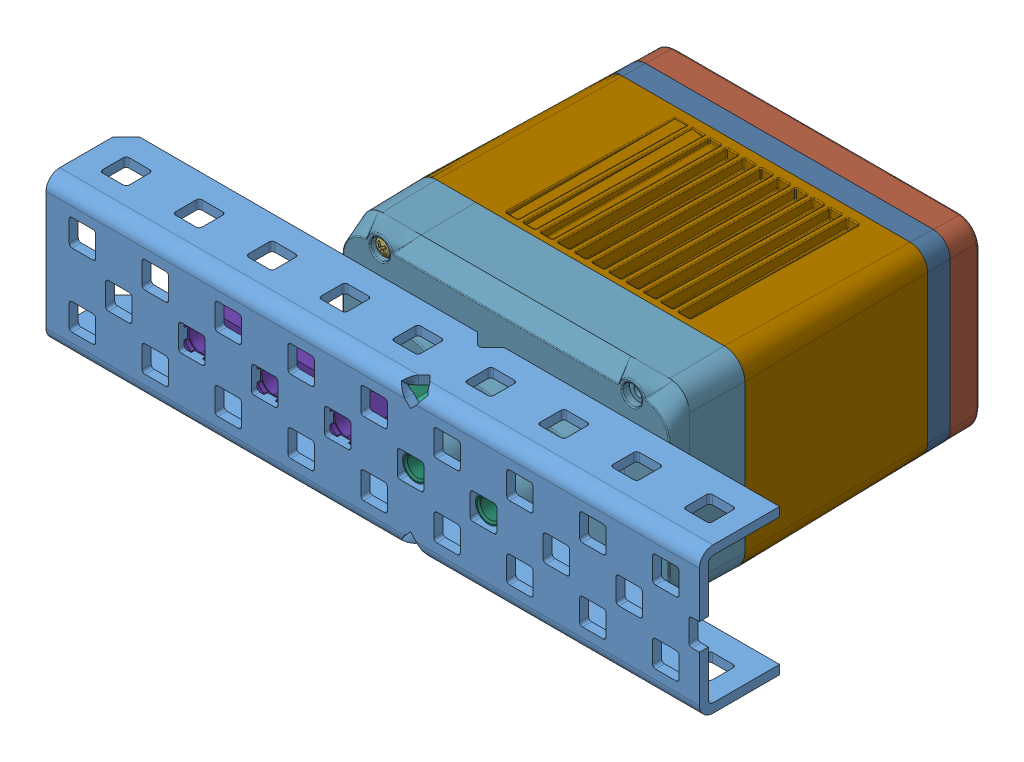
SolidWorks assembly MotorMount1, configuration Default. Lengths in mm.
Overall size (113.79 35.33 73.19).
29 component instances, 17 part files, 6 mates.
Components (placement in the parent):
- 1x2x1x9 Aluminum C-Channel-1: 1x2x1x9 Aluminum C-Channel [Default] at (207.6372 62.1851 92.5266) size (113.79 25.41 13.97)
- V5 Smart Motor (276-4840) 2-1: V5 Smart Motor (276-4840) 2 [Default] at (48.8872 62.1851 46.7518) x (-1 0 0) z (0 0 1) size (59.01 35.33 72.31)
  - V5 Smart Motor (276-4840) 2.step-1: V5 Smart Motor (276-4840) 2.step [Default] at origin size (59.01 35.33 72.31)
    - 276-4840-900 Rev6_Instruction.step-1: 276-4840-900 Rev6_Instruction.step [Default] at (-14.3 0 -17.2) size (52.79 15.94 38.15)
      - 276-4840-901 Rev6.step-1: 276-4840-901 Rev6.step [Default] at (10.75 -10.05 17.8) x (-1 0 0) z (0 0 1) size (49.9 1.6 38.15)
      - 276-4840-902 Rev2.step-1: 276-4840-902 Rev2.step [Default] at (31.25 -9.25 6.2) x (0 0 -1) z (0 -1 0) size (10.35 11.39 15.94)
      - 276-4840-022 Rev4.step-1: 276-4840-022 Rev4.step [Default] at (31.25 -9.25 6.2) x (0 0 -1) z (1 0 0) size (10.26 9.1 5.51)
    - 276-4840-110 Rev10_Instruction.step-1: 276-4840-110 Rev10_Instruction.step [Default] at (12.7 0 14.7) size (35.33 35.33 31.1)
      - 276-4840-061 Rev7_Ring_Gear_Fixed01 .6 Rev3.step-1: 276-4840-061 Rev7_Ring_Gear_Fixed01 .6 Rev3.step [Default] at origin size (28.79 28.39 24.6)
      - 276-4840-018 Rev6.step-1: 276-4840-018 Rev6.step [Default] at (0 0 6.7) x (-0.483174 0.875524 0) z (0 0 1) size (26 26 12.3)
      - 276-4840-059 Rev2.step-1: 276-4840-059 Rev2.step [Default] at (0 0 10.3) size (28.4 28.4 8.5)
      - 276-4840-062 Rev1.step-1: 276-4840-062 Rev1.step [Default] at (-12.1353 8.8168 12.3) x (0.956835 -0.290632 0) z (-0.290632 -0.956835 0) size (3.2 6.56 3.2)
      - 276-4840-062 Rev1.step-2: 276-4840-062 Rev1.step [Default] at (12.1353 8.8168 12.3) x (0.978427 0.206591 0) z (0.206591 -0.978427 0) size (3.2 6.56 3.2)
      - 276-4840-062 Rev1.step-3: 276-4840-062 Rev1.step [Default] at (-12.1353 -8.8168 12.3) x (0.72563 0.688086 0) z (0.688086 -0.72563 0) size (3.2 6.56 3.2)
    - 276-4840-001 Rev38.step-1: 276-4840-001 Rev38.step [Default] at origin size (57.3 33 46.9)
    - 276-4840-005 Rev27.step-1: 276-4840-005 Rev27.step [Default] at (0 0 -17.95) size (56.17 31.87 12.9)
    - 276-4840-004 Rev16.step-1: 276-4840-004 Rev16.step [Default] at (0 0 -19.2) size (56.01 31.71 9.21)
    - 276-4840-015 Rev7.step-1: 276-4840-015 Rev7.step [Default] at (-21.95 14 27.9) x (-0.85131 -0.524663 0) z (-0.524663 0.85131 0) size (3.2 17.55 3.2)
    - 276-4840-015 Rev7.step-2: 276-4840-015 Rev7.step [Default] at (21.95 -14 27.9) x (-0.777574 -0.628792 0) z (-0.628792 0.777574 0) size (3.2 17.55 3.2)
    - 276-4840-015 Rev7.step-3: 276-4840-015 Rev7.step [Default] at (21.95 14 27.9) x (0.476859 0.87898 0) z (0.87898 -0.476859 0) size (3.2 17.55 3.2)
    - 276-4840-009 Rev3.step-1: 276-4840-009 Rev3.step [Default] at (25.45 13.5 15.7) x (0.19987 -0.979823 0) z (-0.979823 -0.19987 0) size (3.4 41.31 4.34)
    - 276-4840-009 Rev3.step-2: 276-4840-009 Rev3.step [Default] at (-25.45 -13.5 15.7) x (-0.998855 0.047836 0) z (0.047836 0.998855 0) size (3.4 41.31 4.34)
    - 276-4840-009 Rev3.step-3: 276-4840-009 Rev3.step [Default] at (25.45 -13.5 15.7) x (-0.975374 0.220559 0) z (0.220559 0.975374 0) size (3.4 41.31 4.34)
    - 276-4840-009 Rev3.step-4: 276-4840-009 Rev3.step [Default] at (-25.45 13.5 15.7) x (-0.922256 0.38658 0) z (0.38658 0.922256 0) size (3.4 41.31 4.34)
    - 276-4840-003 Rev27.step-1: 276-4840-003 Rev27.step [Default] at (0 0 16.2) size (57.3 33 28.01)
    - 276-4840-043 Rev8.step-1: 276-4840-043 Rev8.step [Default] at (-12.7 0 36.2) x (-0.5 -0.866025 0) z (-0.866025 0.5 0) size (6.3 15.2 7.21)
    - 276-4840-043 Rev8.step-2: 276-4840-043 Rev8.step [Default] at (0 0 36.2) x (-0.5 -0.866025 0) z (-0.866025 0.5 0) size (6.3 15.2 7.21)
    - 276-4840-025 Rev19.step-1: 276-4840-025 Rev19.step [Default] at (12.7 0 -22.63) x (-0.993315 0.115437 0) z (0 0 1) size (14.82 14.83 35.18)
- Flat Bearing (276-1209)-1: Flat Bearing (276-1209) [Default] at (-2.9288 74.8851 1.9756) x (0 0 1) z (0 1 0) size (7.04 35.56 10.16)
Mates (geometry in assembly coordinates):
- Coincident1: coincident anti-aligned: plane of 1x2x1x9 Aluminum C-Channel-1 through (-14.1128 40.2648 90.9518) normal (0 0 -1); plane of V5 Smart Motor (276-4840) 2-1/V5 Smart Motor (276-4840) 2.step-1/276-4840-003 Rev27.step-1 through (48.8872 62.1851 90.9518) normal (0 0 1)
- Concentric1: concentric aligned: circle of 1x2x1x9 Aluminum C-Channel-1; circle of V5 Smart Motor (276-4840) 2-1/V5 Smart Motor (276-4840) 2.step-1/276-4840-003 Rev27.step-1
- Parallel1: parallel: plane of 1x2x1x9 Aluminum C-Channel-1 through (-14.1128 74.8851 124.8853) normal (0 1 0); line of V5 Smart Motor (276-4840) 2-1/V5 Smart Motor (276-4840) 2.step-1/276-4840-003 Rev27.step-1 through (68.4145 76.5641 75.9518) axis (-1 0 0)
- Coincident3: coincident anti-aligned: plane of 1x2x1x9 Aluminum C-Channel-1 through (-14.1128 40.2648 90.9518) normal (0 0 -1); plane of Flat Bearing (276-1209)-1 through (41.2709 57.1014 90.9518) normal (0 0 1)
- Concentric2: concentric aligned: cylinder of 1x2x1x9 Aluminum C-Channel-1; cylinder of Flat Bearing (276-1209)-1 through (36.1872 62.1851 84.6018) axis (0 0 1) radius 2.1209
- Parallel2: parallel: plane of 1x2x1x9 Aluminum C-Channel-1 through (-14.1128 73.3103 124.8853) normal (0 -1 0); line of Flat Bearing (276-1209)-1 through (8.2457 67.2651 90.9518) axis (1 0 0)
